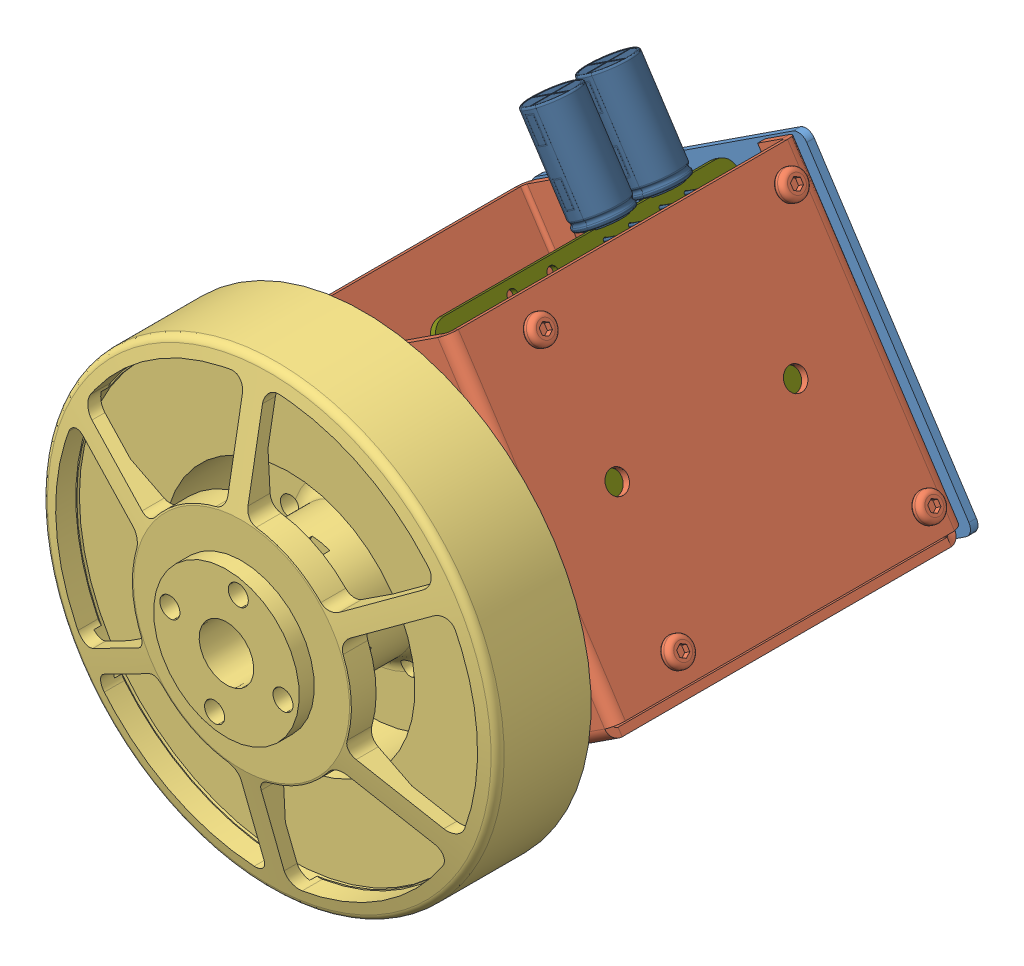
SolidWorks assembly 装配体1, configuration 默认. Lengths in mm.
Overall size (125.4 125.4 105.52).
333 component instances, 38 part files, 34 mates.
Components (placement in the parent):
- 后面板-1: 后面板 [默认] at (-110.0598 38.3936 -13.6207) x (-0.837169 -0.546944 0) z (0 0 -1) size (65 63 1.5)
- 电机架-钣金-1: 电机架-钣金 [默认] at (-110.4773 39.0327 57.0038) x (-0.837169 -0.546944 0) z (0.546944 -0.837169 0) size (65 70 63)
- bldc-motor-A12-1: bldc-motor-A12 [默认] at (-110.4773 39.0327 57.0038) x (-0.837169 -0.546944 0) z (-0.546944 0.837169 0) size (90.6 34.9 90.6)
- simple_bldc.step-1: simple_bldc.step [默认] at (-80.5102 22.4176 -12.7962) x (0 0 1) z (-0.837169 -0.546944 0) size (60.6 79.73 16.29)
  - JST_PH_B6B-PH-K_1x06_P2.00mm_Vertical.step-1: JST_PH_B6B-PH-K_1x06_P2.00mm_Vertical.step [默认] at (24 3 1.25) x (-1 0 0) z (0 0 1) size (13.9 4.55 9.4)
    - SOLID.step-1: SOLID.step [默认] at origin size (13.9 4.55 9.4)
  - SOT-363_SC-70-6.step-1: SOT-363_SC-70-6.step [默认] at (22.4536 8.4836 1.25) size (2 2 1.05)
    - SOLID-0.step-1: SOLID-0.step [默认] at origin size (2 2 1.05)
  - C_0402_1005Metric.step-1: C_0402_1005Metric.step [默认] at (10.668 38.1508 1.25) x (0 -1 0) z (0 0 1) size (1 0.5 0.5)
    - SOLID-1.step-1: SOLID-1.step [默认] at origin size (1 0.5 0.5)
  - PinHeader_1x06_P1.27mm_Vertical.step-1: PinHeader_1x06_P1.27mm_Vertical.step [默认] at (16.9418 25.5778 1.25) size (2.1 7.62 6.3)
    - SOLID-2.step-1: SOLID-2.step [默认] at origin size (2.1 7.62 6.3)
  - C_1206_3216Metric.step-1: C_1206_3216Metric.step [默认] at (7.75 37.6 1.25) size (3.2 1.6 1.6)
    - SOLID-3.step-1: SOLID-3.step [默认] at origin size (3.2 1.6 1.6)
  - LED_0603_1608Metric.step-1: LED_0603_1608Metric.step [默认] at (16.2574 49.0188 1.25) x (0 -1 0) z (0 0 1) size (1.6 0.8 1.1)
    - SOLID-4.step-1: SOLID-4.step [默认] at origin size (1.6 0.8 1.1)
  - SOIC-8_3.9x4.9mm_P1.27mm.step-1: SOIC-8_3.9x4.9mm_P1.27mm.step [默认] at (24.8434 32.3337 1.25) x (0 1 0) z (0 0 1) size (6 4.9 1.75)
    - SOLID-5.step-1: SOLID-5.step [默认] at origin size (6 4.9 1.75)
  - TO-252-5_TabPin3.step-1: TO-252-5_TabPin3.step [默认] at (11.55 45.55 1.25) x (0 1 0) z (0 0 1) size (9.9 6.5 2.32)
    - SOLID-6.step-1: SOLID-6.step [默认] at origin size (9.9 6.5 2.32)
  - R_0402_1005Metric.step-1: R_0402_1005Metric.step [默认] at (25.0698 27.559 1.25) x (0 1 0) z (0 0 1) size (1 0.5 0.35)
    - SOLID-7.step-1: SOLID-7.step [默认] at origin size (1 0.5 0.35)
  - R_0402_1005Metric.step-2: R_0402_1005Metric.step [默认] at (24.003 27.559 1.25) x (0 1 0) z (0 0 1) size (1 0.5 0.35)
    - SOLID-7.step-1: SOLID-7.step [默认] at origin size (1 0.5 0.35)
  - R_0402_1005Metric.step-3: R_0402_1005Metric.step [默认] at (16.2574 46.6188 1.25) x (0 -1 0) z (0 0 1) size (1 0.5 0.35)
    - SOLID-7.step-1: SOLID-7.step [默认] at origin size (1 0.5 0.35)
  - R_0402_1005Metric.step-4: R_0402_1005Metric.step [默认] at (21.3868 36.8046 1.25) size (1 0.5 0.35)
    - SOLID-7.step-1: SOLID-7.step [默认] at origin size (1 0.5 0.35)
  - R_0402_1005Metric.step-5: R_0402_1005Metric.step [默认] at (13.7 38.15 1.25) x (0 1 0) z (0 0 1) size (1 0.5 0.35)
    - SOLID-7.step-1: SOLID-7.step [默认] at origin size (1 0.5 0.35)
  - DFN-8-1EP_6x5mm_Pitch1.27mm.step-1: DFN-8-1EP_6x5mm_Pitch1.27mm.step [默认] at (18.0213 44.6278 -0.05) x (1 0 0) z (0 0 -1) size (6 4.9 1.1)
    - SOLID-8.step-1: SOLID-8.step [默认] at origin size (6 4.9 1.1)
  - PinHeader_1x03_P2.54mm_Vertical.step-1: PinHeader_1x03_P2.54mm_Vertical.step [默认] at (39.5 3 1.25) x (0 1 0) z (0 0 1) size (2.54 7.62 11.54)
    - SOLID-9.step-1: SOLID-9.step [默认] at origin size (2.54 7.62 11.54)
  - D_SOD-123.step-1: D_SOD-123.step [默认] at (20.9804 33.6677 1.25) x (0 -1 0) z (0 0 1) size (3.8 1.6 1.25)
    - SOLID-10.step-1: SOLID-10.step [默认] at origin size (3.8 1.6 1.25)
  - C_0603_1608Metric.step-1: C_0603_1608Metric.step [默认] at (24.003 36.7665 1.25) size (1.6 0.8 0.8)
    - SOLID-11.step-1: SOLID-11.step [默认] at origin size (1.6 0.8 0.8)
  - C_0402_1005Metric.step-2: C_0402_1005Metric.step [默认] at (21.5392 29.6672 1.25) x (0 -1 0) z (0 0 1) size (1 0.5 0.5)
    - SOLID-1.step-1: SOLID-1.step [默认] at origin size (1 0.5 0.5)
  - C_1206_3216Metric.step-2: C_1206_3216Metric.step [默认] at (3.1 37.6 1.25) x (-1 0 0) z (0 0 1) size (3.2 1.6 1.6)
    - SOLID-3.step-1: SOLID-3.step [默认] at origin size (3.2 1.6 1.6)
  - C_0603_1608Metric.step-2: C_0603_1608Metric.step [默认] at (33.3913 36.7634 1.25) size (1.6 0.8 0.8)
    - SOLID-11.step-1: SOLID-11.step [默认] at origin size (1.6 0.8 0.8)
  - C_0402_1005Metric.step-3: C_0402_1005Metric.step [默认] at (30.8413 29.5634 1.25) x (0 -1 0) z (0 0 1) size (1 0.5 0.5)
    - SOLID-1.step-1: SOLID-1.step [默认] at origin size (1 0.5 0.5)
  - R_0402_1005Metric.step-6: R_0402_1005Metric.step [默认] at (41.175 7.6905 1.25) x (-1 0 0) z (0 0 1) size (1 0.5 0.35)
    - SOLID-7.step-1: SOLID-7.step [默认] at origin size (1 0.5 0.35)
  - C_0603_1608Metric.step-3: C_0603_1608Metric.step [默认] at (15.0622 33.2068 1.25) x (-1 0 0) z (0 0 1) size (1.6 0.8 0.8)
    - SOLID-11.step-1: SOLID-11.step [默认] at origin size (1.6 0.8 0.8)
  - C_1206_3216Metric.step-3: C_1206_3216Metric.step [默认] at (1.95 32.15 1.25) x (0 1 0) z (0 0 1) size (3.2 1.6 1.6)
    - SOLID-3.step-1: SOLID-3.step [默认] at origin size (3.2 1.6 1.6)
  - C_1206_3216Metric.step-4: C_1206_3216Metric.step [默认] at (3.1 35.5 1.25) x (-1 0 0) z (0 0 1) size (3.2 1.6 1.6)
    - SOLID-3.step-1: SOLID-3.step [默认] at origin size (3.2 1.6 1.6)
  - C_0603_1608Metric.step-4: C_0603_1608Metric.step [默认] at (15.0622 31.7844 1.25) x (-1 0 0) z (0 0 1) size (1.6 0.8 0.8)
    - SOLID-11.step-1: SOLID-11.step [默认] at origin size (1.6 0.8 0.8)
  - DFN-8-1EP_6x5mm_Pitch1.27mm.step-2: DFN-8-1EP_6x5mm_Pitch1.27mm.step [默认] at (54.7116 46.99 1.25) x (0 1 0) z (0 0 1) size (6 4.9 1.1)
    - SOLID-8.step-1: SOLID-8.step [默认] at origin size (6 4.9 1.1)
  - DFN-8-1EP_6x5mm_Pitch1.27mm.step-3: DFN-8-1EP_6x5mm_Pitch1.27mm.step [默认] at (48.7172 46.99 1.25) x (0 -1 0) z (0 0 1) size (6 4.9 1.1)
    - SOLID-8.step-1: SOLID-8.step [默认] at origin size (6 4.9 1.1)
  - DFN-8-1EP_6x5mm_Pitch1.27mm.step-4: DFN-8-1EP_6x5mm_Pitch1.27mm.step [默认] at (41.0972 46.9392 1.25) x (0 1 0) z (0 0 1) size (6 4.9 1.1)
    - SOLID-8.step-1: SOLID-8.step [默认] at origin size (6 4.9 1.1)
  - DFN-8-1EP_6x5mm_Pitch1.27mm.step-5: DFN-8-1EP_6x5mm_Pitch1.27mm.step [默认] at (35.1028 46.9392 1.25) x (0 -1 0) z (0 0 1) size (6 4.9 1.1)
    - SOLID-8.step-1: SOLID-8.step [默认] at origin size (6 4.9 1.1)
  - DFN-8-1EP_6x5mm_Pitch1.27mm.step-6: DFN-8-1EP_6x5mm_Pitch1.27mm.step [默认] at (27.6352 46.9392 1.25) x (0 1 0) z (0 0 1) size (6 4.9 1.1)
    - SOLID-8.step-1: SOLID-8.step [默认] at origin size (6 4.9 1.1)
  - DFN-8-1EP_6x5mm_Pitch1.27mm.step-7: DFN-8-1EP_6x5mm_Pitch1.27mm.step [默认] at (21.6408 46.9392 1.25) x (0 -1 0) z (0 0 1) size (6 4.9 1.1)
    - SOLID-8.step-1: SOLID-8.step [默认] at origin size (6 4.9 1.1)
  - D_SMA.step-1: D_SMA.step [默认] at (15.3924 28.9904 1.25) size (5 2.7 2.22)
    - SOLID-12.step-1: SOLID-12.step [默认] at origin size (5 2.7 2.22)
  - JST_PH_B4B-PH-K_1x04_P2.00mm_Vertical.step-1: JST_PH_B4B-PH-K_1x04_P2.00mm_Vertical.step [默认] at (35 3 1.25) x (-1 0 0) z (0 0 1) size (9.9 4.55 9.4)
    - SOLID-13.step-1: SOLID-13.step [默认] at origin size (9.9 4.55 9.4)
  - SOT-23-6.step-1: SOT-23-6.step [默认] at (11.0744 16.6878 1.25) size (2.8 2.9 1.55)
    - SOLID-14.step-1: SOLID-14.step [默认] at origin size (2.8 2.9 1.55)
  - D_SOD-123.step-2: D_SOD-123.step [默认] at (6.55 10.55 1.25) size (3.8 1.6 1.25)
    - SOLID-10.step-1: SOLID-10.step [默认] at origin size (3.8 1.6 1.25)
  - PinSocket_1x02_P2.54mm_Vertical.step-1: PinSocket_1x02_P2.54mm_Vertical.step [默认] at (48.5 2.5 1.25) x (-1 0 0) z (0 0 1) size (2.54 5.08 10.1)
    - SOLID-15.step-1: SOLID-15.step [默认] at origin size (2.54 5.08 10.1)
  - R_0402_1005Metric.step-7: R_0402_1005Metric.step [默认] at (4.35 33.7 1.25) size (1 0.5 0.35)
    - SOLID-7.step-1: SOLID-7.step [默认] at origin size (1 0.5 0.35)
  - R_0402_1005Metric.step-8: R_0402_1005Metric.step [默认] at (20.5 11 1.25) size (1 0.5 0.35)
    - SOLID-7.step-1: SOLID-7.step [默认] at origin size (1 0.5 0.35)
  - SOIC-8_3.9x4.9mm_P1.27mm.step-2: SOIC-8_3.9x4.9mm_P1.27mm.step [默认] at (41.15 12.1279 1.25) x (0 -1 0) z (0 0 1) size (6 4.9 1.75)
    - SOLID-5.step-1: SOLID-5.step [默认] at origin size (6 4.9 1.75)
  - LQFP-64_10x10mm_P0.5mm.step-1: LQFP-64_10x10mm_P0.5mm.step [默认] at (28.698 16.1455 1.25) x (0 -1 0) z (0 0 1) size (12 12 1.5)
    - SOLID-16.step-1: SOLID-16.step [默认] at origin size (12 12 1.5)
  - SOT-23-6.step-2: SOT-23-6.step [默认] at (7.239 32.3432 1.25) x (-1 0 0) z (0 0 1) size (2.8 2.9 1.55)
    - SOLID-14.step-1: SOLID-14.step [默认] at origin size (2.8 2.9 1.55)
  - C_1206_3216Metric.step-5: C_1206_3216Metric.step [默认] at (37.8884 45.2528 -0.05) x (0 1 0) z (0 0 -1) size (3.2 1.6 1.6)
    - SOLID-3.step-1: SOLID-3.step [默认] at origin size (3.2 1.6 1.6)
  - C_1206_3216Metric.step-6: C_1206_3216Metric.step [默认] at (26.5939 45.2528 -0.05) x (0 1 0) z (0 0 -1) size (3.2 1.6 1.6)
    - SOLID-3.step-1: SOLID-3.step [默认] at origin size (3.2 1.6 1.6)
  - C_1206_3216Metric.step-7: C_1206_3216Metric.step [默认] at (51.0964 46.3704 -0.05) x (-1 0 0) z (0 0 -1) size (3.2 1.6 1.6)
    - SOLID-3.step-1: SOLID-3.step [默认] at origin size (3.2 1.6 1.6)
  - C_1206_3216Metric.step-8: C_1206_3216Metric.step [默认] at (30.9288 45.2528 -0.05) x (0 1 0) z (0 0 -1) size (3.2 1.6 1.6)
    - SOLID-3.step-1: SOLID-3.step [默认] at origin size (3.2 1.6 1.6)
  - C_1206_3216Metric.step-9: C_1206_3216Metric.step [默认] at (24.4264 45.2528 -0.05) x (0 1 0) z (0 0 -1) size (3.2 1.6 1.6)
    - SOLID-3.step-1: SOLID-3.step [默认] at origin size (3.2 1.6 1.6)
  - C_1206_3216Metric.step-10: C_1206_3216Metric.step [默认] at (51.0964 44.1352 -0.05) x (-1 0 0) z (0 0 -1) size (3.2 1.6 1.6)
    - SOLID-3.step-1: SOLID-3.step [默认] at origin size (3.2 1.6 1.6)
  - C_1206_3216Metric.step-11: C_1206_3216Metric.step [默认] at (42.2233 45.2528 -0.05) x (0 1 0) z (0 0 -1) size (3.2 1.6 1.6)
    - SOLID-3.step-1: SOLID-3.step [默认] at origin size (3.2 1.6 1.6)
  - C_1206_3216Metric.step-12: C_1206_3216Metric.step [默认] at (28.7613 45.2528 -0.05) x (0 1 0) z (0 0 -1) size (3.2 1.6 1.6)
    - SOLID-3.step-1: SOLID-3.step [默认] at origin size (3.2 1.6 1.6)
  - C_1206_3216Metric.step-13: C_1206_3216Metric.step [默认] at (40.0559 45.2528 -0.05) x (0 1 0) z (0 0 -1) size (3.2 1.6 1.6)
    - SOLID-3.step-1: SOLID-3.step [默认] at origin size (3.2 1.6 1.6)
  - C_1206_3216Metric.step-14: C_1206_3216Metric.step [默认] at (44.3908 45.2528 -0.05) x (0 1 0) z (0 0 -1) size (3.2 1.6 1.6)
    - SOLID-3.step-1: SOLID-3.step [默认] at origin size (3.2 1.6 1.6)
  - C_0402_1005Metric.step-4: C_0402_1005Metric.step [默认] at (25.4 24.3332 1.25) x (0 -1 0) z (0 0 1) size (1 0.5 0.5)
    - SOLID-1.step-1: SOLID-1.step [默认] at origin size (1 0.5 0.5)
  - C_1206_3216Metric.step-15: C_1206_3216Metric.step [默认] at (46.6852 41.0972 1.25) x (0 1 0) z (0 0 1) size (3.2 1.6 1.6)
    - SOLID-3.step-1: SOLID-3.step [默认] at origin size (3.2 1.6 1.6)
  - C_1206_3216Metric.step-16: C_1206_3216Metric.step [默认] at (33.2232 41.0464 1.25) x (0 1 0) z (0 0 1) size (3.2 1.6 1.6)
    - SOLID-3.step-1: SOLID-3.step [默认] at origin size (3.2 1.6 1.6)
  - C_1206_3216Metric.step-17: C_1206_3216Metric.step [默认] at (19.7104 41.0464 1.25) x (0 1 0) z (0 0 1) size (3.2 1.6 1.6)
    - SOLID-3.step-1: SOLID-3.step [默认] at origin size (3.2 1.6 1.6)
  - C_1206_3216Metric.step-18: C_1206_3216Metric.step [默认] at (49.008 41.12 1.25) x (0 1 0) z (0 0 1) size (3.2 1.6 1.6)
    - SOLID-3.step-1: SOLID-3.step [默认] at origin size (3.2 1.6 1.6)
  - C_1206_3216Metric.step-19: C_1206_3216Metric.step [默认] at (22.0076 41.0825 1.25) x (0 1 0) z (0 0 1) size (3.2 1.6 1.6)
    - SOLID-3.step-1: SOLID-3.step [默认] at origin size (3.2 1.6 1.6)
  - C_1206_3216Metric.step-20: C_1206_3216Metric.step [默认] at (35.4864 41.0708 1.25) x (0 1 0) z (0 0 1) size (3.2 1.6 1.6)
    - SOLID-3.step-1: SOLID-3.step [默认] at origin size (3.2 1.6 1.6)
  - R_0402_1005Metric.step-9: R_0402_1005Metric.step [默认] at (54.5846 36.7411 1.25) x (-1 0 0) z (0 0 1) size (1 0.5 0.35)
    - SOLID-7.step-1: SOLID-7.step [默认] at origin size (1 0.5 0.35)
  - R_0402_1005Metric.step-10: R_0402_1005Metric.step [默认] at (48.4378 36.7919 1.25) x (-1 0 0) z (0 0 1) size (1 0.5 0.35)
    - SOLID-7.step-1: SOLID-7.step [默认] at origin size (1 0.5 0.35)
  - R_0402_1005Metric.step-11: R_0402_1005Metric.step [默认] at (45.6184 36.7411 1.25) x (-1 0 0) z (0 0 1) size (1 0.5 0.35)
    - SOLID-7.step-1: SOLID-7.step [默认] at origin size (1 0.5 0.35)
  - R_0402_1005Metric.step-12: R_0402_1005Metric.step [默认] at (39.2684 36.7919 1.25) x (-1 0 0) z (0 0 1) size (1 0.5 0.35)
    - SOLID-7.step-1: SOLID-7.step [默认] at origin size (1 0.5 0.35)
  - R_0402_1005Metric.step-13: R_0402_1005Metric.step [默认] at (36.4871 36.7284 1.25) x (-1 0 0) z (0 0 1) size (1 0.5 0.35)
    - SOLID-7.step-1: SOLID-7.step [默认] at origin size (1 0.5 0.35)
  - R_0402_1005Metric.step-14: R_0402_1005Metric.step [默认] at (30.4165 36.8046 1.25) x (-1 0 0) z (0 0 1) size (1 0.5 0.35)
    - SOLID-7.step-1: SOLID-7.step [默认] at origin size (1 0.5 0.35)
  - SOIC-8_3.9x4.9mm_P1.27mm.step-3: SOIC-8_3.9x4.9mm_P1.27mm.step [默认] at (52.3494 32.3499 1.25) x (0 1 0) z (0 0 1) size (6 4.9 1.75)
    - SOLID-5.step-1: SOLID-5.step [默认] at origin size (6 4.9 1.75)
  - L_Bourns-SRN4018.step-1: L_Bourns-SRN4018.step [默认] at (11.4 32.8 1.25) size (4 4.09 1.8)
    - COMPOUND.step-1: COMPOUND.step [默认] at origin size (4 4.09 1.8)
  - D_SOD-123.step-3: D_SOD-123.step [默认] at (48.4886 33.6423 1.25) x (0 -1 0) z (0 0 1) size (3.8 1.6 1.25)
    - SOLID-10.step-1: SOLID-10.step [默认] at origin size (3.8 1.6 1.25)
  - D_SOD-123.step-4: D_SOD-123.step [默认] at (39.4208 33.6931 1.25) x (0 -1 0) z (0 0 1) size (3.8 1.6 1.25)
    - SOLID-10.step-1: SOLID-10.step [默认] at origin size (3.8 1.6 1.25)
  - D_SOD-123.step-5: D_SOD-123.step [默认] at (30.2641 33.7058 1.25) x (0 -1 0) z (0 0 1) size (3.8 1.6 1.25)
    - SOLID-10.step-1: SOLID-10.step [默认] at origin size (3.8 1.6 1.25)
  - SOIC-8_3.9x4.9mm_P1.27mm.step-4: SOIC-8_3.9x4.9mm_P1.27mm.step [默认] at (43.3324 32.3215 1.25) x (0 1 0) z (0 0 1) size (6 4.9 1.75)
    - SOLID-5.step-1: SOLID-5.step [默认] at origin size (6 4.9 1.75)
  - SOIC-8_3.9x4.9mm_P1.27mm.step-5: SOIC-8_3.9x4.9mm_P1.27mm.step [默认] at (34.1249 32.3342 1.25) x (0 1 0) z (0 0 1) size (6 4.9 1.75)
    - SOLID-5.step-1: SOLID-5.step [默认] at origin size (6 4.9 1.75)
  - SOIC-14_3.9x8.7mm_P1.27mm.step-1: SOIC-14_3.9x8.7mm_P1.27mm.step [默认] at (50.625 22.3111 1.25) x (-1 0 0) z (0 0 1) size (6 8.7 1.75)
    - SOLID-17.step-1: SOLID-17.step [默认] at origin size (6 8.7 1.75)
  - R_0402_1005Metric.step-15: R_0402_1005Metric.step [默认] at (27.2288 26.2382 1.25) x (0 -1 0) z (0 0 1) size (1 0.5 0.35)
    - SOLID-7.step-1: SOLID-7.step [默认] at origin size (1 0.5 0.35)
  - R_0402_1005Metric.step-16: R_0402_1005Metric.step [默认] at (46.863 29.6418 1.25) x (0 -1 0) z (0 0 1) size (1 0.5 0.35)
    - SOLID-7.step-1: SOLID-7.step [默认] at origin size (1 0.5 0.35)
  - R_0402_1005Metric.step-17: R_0402_1005Metric.step [默认] at (47.8028 29.6418 1.25) x (0 -1 0) z (0 0 1) size (1 0.5 0.35)
    - SOLID-7.step-1: SOLID-7.step [默认] at origin size (1 0.5 0.35)
  - R_0402_1005Metric.step-18: R_0402_1005Metric.step [默认] at (37.7063 29.6799 1.25) x (0 -1 0) z (0 0 1) size (1 0.5 0.35)
    - SOLID-7.step-1: SOLID-7.step [默认] at origin size (1 0.5 0.35)
  - R_0402_1005Metric.step-19: R_0402_1005Metric.step [默认] at (38.6588 29.6799 1.25) x (0 -1 0) z (0 0 1) size (1 0.5 0.35)
    - SOLID-7.step-1: SOLID-7.step [默认] at origin size (1 0.5 0.35)
  - R_0402_1005Metric.step-20: R_0402_1005Metric.step [默认] at (28.4734 29.5783 1.25) x (0 -1 0) z (0 0 1) size (1 0.5 0.35)
    - SOLID-7.step-1: SOLID-7.step [默认] at origin size (1 0.5 0.35)
  - R_0402_1005Metric.step-21: R_0402_1005Metric.step [默认] at (29.4513 29.591 1.25) x (0 -1 0) z (0 0 1) size (1 0.5 0.35)
    - SOLID-7.step-1: SOLID-7.step [默认] at origin size (1 0.5 0.35)
  - R_0402_1005Metric.step-22: R_0402_1005Metric.step [默认] at (45.5704 23.3271 1.25) x (-1 0 0) z (0 0 1) size (1 0.5 0.35)
    - SOLID-7.step-1: SOLID-7.step [默认] at origin size (1 0.5 0.35)
  - R_0402_1005Metric.step-23: R_0402_1005Metric.step [默认] at (45.5704 24.2415 1.25) x (-1 0 0) z (0 0 1) size (1 0.5 0.35)
    - SOLID-7.step-1: SOLID-7.step [默认] at origin size (1 0.5 0.35)
  - R_0402_1005Metric.step-24: R_0402_1005Metric.step [默认] at (55.6232 24.0665 1.25) size (1 0.5 0.35)
    - SOLID-7.step-1: SOLID-7.step [默认] at origin size (1 0.5 0.35)
  - R_0402_1005Metric.step-25: R_0402_1005Metric.step [默认] at (55.6232 24.9555 1.25) size (1 0.5 0.35)
    - SOLID-7.step-1: SOLID-7.step [默认] at origin size (1 0.5 0.35)
  - R_0402_1005Metric.step-26: R_0402_1005Metric.step [默认] at (36.8554 17.3736 1.25) x (-1 0 0) z (0 0 1) size (1 0.5 0.35)
    - SOLID-7.step-1: SOLID-7.step [默认] at origin size (1 0.5 0.35)
  - R_0402_1005Metric.step-27: R_0402_1005Metric.step [默认] at (45.5704 22.3619 1.25) x (-1 0 0) z (0 0 1) size (1 0.5 0.35)
    - SOLID-7.step-1: SOLID-7.step [默认] at origin size (1 0.5 0.35)
  - R_0402_1005Metric.step-28: R_0402_1005Metric.step [默认] at (45.5704 25.1559 1.25) x (-1 0 0) z (0 0 1) size (1 0.5 0.35)
    - SOLID-7.step-1: SOLID-7.step [默认] at origin size (1 0.5 0.35)
  - R_0402_1005Metric.step-29: R_0402_1005Metric.step [默认] at (55.626 23.1775 1.25) x (-1 0 0) z (0 0 1) size (1 0.5 0.35)
    - SOLID-7.step-1: SOLID-7.step [默认] at origin size (1 0.5 0.35)
  - R_0402_1005Metric.step-30: R_0402_1005Metric.step [默认] at (55.626 25.8699 1.25) x (-1 0 0) z (0 0 1) size (1 0.5 0.35)
    - SOLID-7.step-1: SOLID-7.step [默认] at origin size (1 0.5 0.35)
  - R_0402_1005Metric.step-31: R_0402_1005Metric.step [默认] at (45.5704 26.0731 1.25) size (1 0.5 0.35)
    - SOLID-7.step-1: SOLID-7.step [默认] at origin size (1 0.5 0.35)
  - R_0402_1005Metric.step-32: R_0402_1005Metric.step [默认] at (55.626 26.7589 1.25) x (-1 0 0) z (0 0 1) size (1 0.5 0.35)
    - SOLID-7.step-1: SOLID-7.step [默认] at origin size (1 0.5 0.35)
  - R_0402_1005Metric.step-33: R_0402_1005Metric.step [默认] at (55.626 20.4851 1.25) size (1 0.5 0.35)
    - SOLID-7.step-1: SOLID-7.step [默认] at origin size (1 0.5 0.35)
  - R_0402_1005Metric.step-34: R_0402_1005Metric.step [默认] at (55.6288 19.5933 1.25) size (1 0.5 0.35)
    - SOLID-7.step-1: SOLID-7.step [默认] at origin size (1 0.5 0.35)
  - R_0402_1005Metric.step-35: R_0402_1005Metric.step [默认] at (11.6 38.15 1.25) x (0 1 0) z (0 0 1) size (1 0.5 0.35)
    - SOLID-7.step-1: SOLID-7.step [默认] at origin size (1 0.5 0.35)
  - R_0402_1005Metric.step-36: R_0402_1005Metric.step [默认] at (4.3434 31.8606 1.25) x (-1 0 0) z (0 0 1) size (1 0.5 0.35)
    - SOLID-7.step-1: SOLID-7.step [默认] at origin size (1 0.5 0.35)
  - R_0402_1005Metric.step-37: R_0402_1005Metric.step [默认] at (55.626 21.3995 1.25) x (-1 0 0) z (0 0 1) size (1 0.5 0.35)
    - SOLID-7.step-1: SOLID-7.step [默认] at origin size (1 0.5 0.35)
  - R_0402_1005Metric.step-38: R_0402_1005Metric.step [默认] at (12.6 38.15 1.25) x (0 -1 0) z (0 0 1) size (1 0.5 0.35)
    - SOLID-7.step-1: SOLID-7.step [默认] at origin size (1 0.5 0.35)
  - R_0402_1005Metric.step-39: R_0402_1005Metric.step [默认] at (55.6288 18.7071 1.25) size (1 0.5 0.35)
    - SOLID-7.step-1: SOLID-7.step [默认] at origin size (1 0.5 0.35)
  - R_0402_1005Metric.step-40: R_0402_1005Metric.step [默认] at (4.3434 32.775 1.25) size (1 0.5 0.35)
    - SOLID-7.step-1: SOLID-7.step [默认] at origin size (1 0.5 0.35)
  - R_0402_1005Metric.step-41: R_0402_1005Metric.step [默认] at (55.6288 17.8181 1.25) x (-1 0 0) z (0 0 1) size (1 0.5 0.35)
    - SOLID-7.step-1: SOLID-7.step [默认] at origin size (1 0.5 0.35)
  - R_0402_1005Metric.step-42: R_0402_1005Metric.step [默认] at (45.5704 18.6817 1.25) x (-1 0 0) z (0 0 1) size (1 0.5 0.35)
    - SOLID-7.step-1: SOLID-7.step [默认] at origin size (1 0.5 0.35)
  - R_0402_1005Metric.step-43: R_0402_1005Metric.step [默认] at (45.5704 20.5613 1.25) size (1 0.5 0.35)
    - SOLID-7.step-1: SOLID-7.step [默认] at origin size (1 0.5 0.35)
  - R_0402_1005Metric.step-44: R_0402_1005Metric.step [默认] at (20.4724 20.7772 1.25) x (-1 0 0) z (0 0 1) size (1 0.5 0.35)
    - SOLID-7.step-1: SOLID-7.step [默认] at origin size (1 0.5 0.35)
  - R_0402_1005Metric.step-45: R_0402_1005Metric.step [默认] at (36.8554 16.4338 1.25) size (1 0.5 0.35)
    - SOLID-7.step-1: SOLID-7.step [默认] at origin size (1 0.5 0.35)
  - R_0402_1005Metric.step-46: R_0402_1005Metric.step [默认] at (14.6522 12.8757 1.25) x (0 1 0) z (0 0 1) size (1 0.5 0.35)
    - SOLID-7.step-1: SOLID-7.step [默认] at origin size (1 0.5 0.35)
  - R_0402_1005Metric.step-47: R_0402_1005Metric.step [默认] at (16.459 12.8757 1.25) x (0 1 0) z (0 0 1) size (1 0.5 0.35)
    - SOLID-7.step-1: SOLID-7.step [默认] at origin size (1 0.5 0.35)
  - R_0402_1005Metric.step-48: R_0402_1005Metric.step [默认] at (18.2556 12.8757 1.25) x (0 1 0) z (0 0 1) size (1 0.5 0.35)
    - SOLID-7.step-1: SOLID-7.step [默认] at origin size (1 0.5 0.35)
  - R_0402_1005Metric.step-49: R_0402_1005Metric.step [默认] at (14.18 16.2386 1.25) x (-1 0 0) z (0 0 1) size (1 0.5 0.35)
    - SOLID-7.step-1: SOLID-7.step [默认] at origin size (1 0.5 0.35)
  - R_0402_1005Metric.step-50: R_0402_1005Metric.step [默认] at (14.18 17.145 1.25) x (-1 0 0) z (0 0 1) size (1 0.5 0.35)
    - SOLID-7.step-1: SOLID-7.step [默认] at origin size (1 0.5 0.35)
  - R_0402_1005Metric.step-51: R_0402_1005Metric.step [默认] at (26.3144 24.3078 1.25) x (0 -1 0) z (0 0 1) size (1 0.5 0.35)
    - SOLID-7.step-1: SOLID-7.step [默认] at origin size (1 0.5 0.35)
  - R_0402_1005Metric.step-52: R_0402_1005Metric.step [默认] at (16.0528 38.1508 1.25) x (0 -1 0) z (0 0 1) size (1 0.5 0.35)
    - SOLID-7.step-1: SOLID-7.step [默认] at origin size (1 0.5 0.35)
  - HRO_TYPE-C-31-M-12.step-1: HRO_TYPE-C-31-M-12.step [默认] at (-0.6 22 1.25) x (0 -1 0) z (0 0 1) size (8.95 7.9 4.2)
    - SOLID-18.step-1: SOLID-18.step [默认] at origin size (6 4.32 0.61)
    - SOLID-19.step-1: SOLID-19.step [默认] at origin size (6.9 0.99 0.3)
    - SOLID-20.step-1: SOLID-20.step [默认] at origin size (8.95 6.5 3.7)
    - SOLID-21.step-1: SOLID-21.step [默认] at origin size (8.95 7.3 4.2)
  - C_0402_1005Metric.step-5: C_0402_1005Metric.step [默认] at (41.1904 16.4281 1.25) size (1 0.5 0.5)
    - SOLID-1.step-1: SOLID-1.step [默认] at origin size (1 0.5 0.5)
  - C_0402_1005Metric.step-6: C_0402_1005Metric.step [默认] at (34.036 22.2758 1.25) x (-1 0 0) z (0 0 1) size (1 0.5 0.5)
    - SOLID-1.step-1: SOLID-1.step [默认] at origin size (1 0.5 0.5)
  - C_0402_1005Metric.step-7: C_0402_1005Metric.step [默认] at (20.4724 18.8722 1.25) size (1 0.5 0.5)
    - SOLID-1.step-1: SOLID-1.step [默认] at origin size (1 0.5 0.5)
  - C_0402_1005Metric.step-8: C_0402_1005Metric.step [默认] at (20.4978 12.0142 1.25) size (1 0.5 0.5)
    - SOLID-1.step-1: SOLID-1.step [默认] at origin size (1 0.5 0.5)
  - C_0402_1005Metric.step-9: C_0402_1005Metric.step [默认] at (34.2392 9.8044 1.25) x (-1 0 0) z (0 0 1) size (1 0.5 0.5)
    - SOLID-1.step-1: SOLID-1.step [默认] at origin size (1 0.5 0.5)
  - C_0402_1005Metric.step-10: C_0402_1005Metric.step [默认] at (36.83 19.7866 1.25) x (-1 0 0) z (0 0 1) size (1 0.5 0.5)
    - SOLID-1.step-1: SOLID-1.step [默认] at origin size (1 0.5 0.5)
  - C_0402_1005Metric.step-11: C_0402_1005Metric.step [默认] at (28.448 26.2382 1.25) x (0 1 0) z (0 0 1) size (1 0.5 0.5)
    - SOLID-1.step-1: SOLID-1.step [默认] at origin size (1 0.5 0.5)
  - C_0402_1005Metric.step-12: C_0402_1005Metric.step [默认] at (24.4856 24.3332 1.25) x (0 -1 0) z (0 0 1) size (1 0.5 0.5)
    - SOLID-1.step-1: SOLID-1.step [默认] at origin size (1 0.5 0.5)
  - C_0402_1005Metric.step-13: C_0402_1005Metric.step [默认] at (28.448 24.3078 1.25) x (0 -1 0) z (0 0 1) size (1 0.5 0.5)
    - SOLID-1.step-1: SOLID-1.step [默认] at origin size (1 0.5 0.5)
  - C_0402_1005Metric.step-14: C_0402_1005Metric.step [默认] at (35.7632 26.2128 1.25) x (0 1 0) z (0 0 1) size (1 0.5 0.5)
    - SOLID-1.step-1: SOLID-1.step [默认] at origin size (1 0.5 0.5)
  - C_0402_1005Metric.step-15: C_0402_1005Metric.step [默认] at (34.2392 8.8646 1.25) size (1 0.5 0.5)
    - SOLID-1.step-1: SOLID-1.step [默认] at origin size (1 0.5 0.5)
  - C_0402_1005Metric.step-16: C_0402_1005Metric.step [默认] at (20.498 12.9455 1.25) x (-1 0 0) z (0 0 1) size (1 0.5 0.5)
    - SOLID-1.step-1: SOLID-1.step [默认] at origin size (1 0.5 0.5)
  - C_0603_1608Metric.step-5: C_0603_1608Metric.step [默认] at (51.689 36.7919 1.25) size (1.6 0.8 0.8)
    - SOLID-11.step-1: SOLID-11.step [默认] at origin size (1.6 0.8 0.8)
  - C_0402_1005Metric.step-17: C_0402_1005Metric.step [默认] at (49.1236 29.6164 1.25) x (0 -1 0) z (0 0 1) size (1 0.5 0.5)
    - SOLID-1.step-1: SOLID-1.step [默认] at origin size (1 0.5 0.5)
  - C_0603_1608Metric.step-6: C_0603_1608Metric.step [默认] at (42.672 36.7919 1.25) size (1.6 0.8 0.8)
    - SOLID-11.step-1: SOLID-11.step [默认] at origin size (1.6 0.8 0.8)
  - C_0402_1005Metric.step-18: C_0402_1005Metric.step [默认] at (44.148 23.7843 1.25) x (0 -1 0) z (0 0 1) size (1 0.5 0.5)
    - SOLID-1.step-1: SOLID-1.step [默认] at origin size (1 0.5 0.5)
  - C_0402_1005Metric.step-19: C_0402_1005Metric.step [默认] at (56.9976 24.4983 1.25) x (0 1 0) z (0 0 1) size (1 0.5 0.5)
    - SOLID-1.step-1: SOLID-1.step [默认] at origin size (1 0.5 0.5)
  - C_0402_1005Metric.step-20: C_0402_1005Metric.step [默认] at (40.0812 29.6799 1.25) x (0 -1 0) z (0 0 1) size (1 0.5 0.5)
    - SOLID-1.step-1: SOLID-1.step [默认] at origin size (1 0.5 0.5)
  - C_0402_1005Metric.step-21: C_0402_1005Metric.step [默认] at (44.1452 25.6159 1.25) x (0 1 0) z (0 0 1) size (1 0.5 0.5)
    - SOLID-1.step-1: SOLID-1.step [默认] at origin size (1 0.5 0.5)
  - C_0402_1005Metric.step-22: C_0402_1005Metric.step [默认] at (56.9976 26.3017 1.25) x (0 1 0) z (0 0 1) size (1 0.5 0.5)
    - SOLID-1.step-1: SOLID-1.step [默认] at origin size (1 0.5 0.5)
  - C_0402_1005Metric.step-23: C_0402_1005Metric.step [默认] at (55.626 22.2885 1.25) x (-1 0 0) z (0 0 1) size (1 0.5 0.5)
    - SOLID-1.step-1: SOLID-1.step [默认] at origin size (1 0.5 0.5)
  - C_0402_1005Metric.step-24: C_0402_1005Metric.step [默认] at (57.0004 20.0505 1.25) x (0 1 0) z (0 0 1) size (1 0.5 0.5)
    - SOLID-1.step-1: SOLID-1.step [默认] at origin size (1 0.5 0.5)
  - C_0402_1005Metric.step-25: C_0402_1005Metric.step [默认] at (4.3434 30.9462 1.25) x (-1 0 0) z (0 0 1) size (1 0.5 0.5)
    - SOLID-1.step-1: SOLID-1.step [默认] at origin size (1 0.5 0.5)
  - C_0402_1005Metric.step-26: C_0402_1005Metric.step [默认] at (56.9976 18.2499 1.25) x (0 -1 0) z (0 0 1) size (1 0.5 0.5)
    - SOLID-1.step-1: SOLID-1.step [默认] at origin size (1 0.5 0.5)
  - C_0603_1608Metric.step-7: C_0603_1608Metric.step [默认] at (7.6708 35.2388 1.25) size (1.6 0.8 0.8)
    - SOLID-11.step-1: SOLID-11.step [默认] at origin size (1.6 0.8 0.8)
  - C_0402_1005Metric.step-27: C_0402_1005Metric.step [默认] at (45.5504 19.5989 1.25) x (-1 0 0) z (0 0 1) size (1 0.5 0.5)
    - SOLID-1.step-1: SOLID-1.step [默认] at origin size (1 0.5 0.5)
  - C_0402_1005Metric.step-28: C_0402_1005Metric.step [默认] at (20.464 16.2206 1.25) size (1 0.5 0.5)
    - SOLID-1.step-1: SOLID-1.step [默认] at origin size (1 0.5 0.5)
  - C_0402_1005Metric.step-29: C_0402_1005Metric.step [默认] at (20.4724 19.8374 1.25) x (-1 0 0) z (0 0 1) size (1 0.5 0.5)
    - SOLID-1.step-1: SOLID-1.step [默认] at origin size (1 0.5 0.5)
  - C_0402_1005Metric.step-30: C_0402_1005Metric.step [默认] at (27.2542 24.3078 1.25) x (0 -1 0) z (0 0 1) size (1 0.5 0.5)
    - SOLID-1.step-1: SOLID-1.step [默认] at origin size (1 0.5 0.5)
  - D_SMA.step-2: D_SMA.step [默认] at (4.3 49.35 1.25) x (-1 0 0) z (0 0 1) size (5 2.7 2.22)
    - SOLID-12.step-1: SOLID-12.step [默认] at origin size (5 2.7 2.22)
  - cap_el_horizontal_d10_h20_pitch5_w0.6.step-1: cap_el_horizontal_d10_h20_pitch5_w0.6.step [默认] at (23.55 57.925 -3.5) x (0 -1 0) z (0 0 1) size (22.11 10.01 13.1)
    - SOLID-22.step-1: SOLID-22.step [默认] at origin size (22.11 10.01 13.1)
  - cap_el_horizontal_d10_h20_pitch5_w0.6.step-2: cap_el_horizontal_d10_h20_pitch5_w0.6.step [默认] at (12.4266 57.925 -3.5) x (0 -1 0) z (0 0 1) size (22.11 10.01 13.1)
    - SOLID-22.step-1: SOLID-22.step [默认] at origin size (22.11 10.01 13.1)
  - R_2512_6332Metric.step-1: R_2512_6332Metric.step [默认] at (40.8348 40.7918 1.25) size (6.3 3.2 0.6)
    - SOLID-23.step-1: SOLID-23.step [默认] at origin size (6.3 3.2 0.6)
  - R_2512_6332Metric.step-2: R_2512_6332Metric.step [默认] at (54.3476 40.8502 1.25) size (6.3 3.2 0.6)
    - SOLID-23.step-1: SOLID-23.step [默认] at origin size (6.3 3.2 0.6)
  - C_0603_1608Metric.step-8: C_0603_1608Metric.step [默认] at (11.176 25.663 1.25) x (0 -1 0) z (0 0 1) size (1.6 0.8 0.8)
    - SOLID-11.step-1: SOLID-11.step [默认] at origin size (1.6 0.8 0.8)
  - SOT-223.step-1: SOT-223.step [默认] at (5.9838 27.0848 1.25) x (-1 0 0) z (0 0 1) size (7 6.5 1.7)
    - SOLID-24.step-1: SOLID-24.step [默认] at origin size (7 6.5 1.7)
  - C_0603_1608Metric.step-9: C_0603_1608Metric.step [默认] at (11.176 28.6348 1.25) x (0 1 0) z (0 0 1) size (1.6 0.8 0.8)
    - SOLID-11.step-1: SOLID-11.step [默认] at origin size (1.6 0.8 0.8)
  - R_0603_1608Metric.step-1: R_0603_1608Metric.step [默认] at (17.5514 45.212 1.25) x (0 -1 0) z (0 0 1) size (1.6 0.8 0.45)
    - SOLID-25.step-1: SOLID-25.step [默认] at origin size (1.6 0.8 0.45)
  - LED_0603_1608Metric.step-2: LED_0603_1608Metric.step [默认] at (18.2556 9.8757 1.25) x (0 1 0) z (0 0 1) size (1.6 0.8 1.1)
    - SOLID-4.step-1: SOLID-4.step [默认] at origin size (1.6 0.8 1.1)
  - L_Bourns_SRN6045TA.step-1: L_Bourns_SRN6045TA.step [默认] at (4.1 43.3 1.25) x (0 -1 0) z (0 0 1) size (6 6 4.2)
    - SOLID-26.step-1: SOLID-26.step [默认] at origin size (6 6 4.2)
  - LED_0603_1608Metric.step-3: LED_0603_1608Metric.step [默认] at (14.6522 9.8757 1.25) x (0 1 0) z (0 0 1) size (1.6 0.8 1.1)
    - SOLID-4.step-1: SOLID-4.step [默认] at origin size (1.6 0.8 1.1)
  - Oscillator_SMD_EuroQuartz_XO53-4Pin_5.0x3.2mm.step-1: Oscillator_SMD_EuroQuartz_XO53-4Pin_5.0x3.2mm.step [默认] at (32.1232 25.2308 1.25) x (-1 0 0) z (0 0 1) size (5 3.2 1)
    - SOLID-27.step-1: SOLID-27.step [默认] at origin size (5 3.2 1)
  - LED_0603_1608Metric.step-4: LED_0603_1608Metric.step [默认] at (16.459 9.8757 1.25) x (0 1 0) z (0 0 1) size (1.6 0.8 1.1)
    - SOLID-4.step-1: SOLID-4.step [默认] at origin size (1.6 0.8 1.1)
  - R_2512_6332Metric.step-3: R_2512_6332Metric.step [默认] at (27.3204 40.7852 1.25) size (6.3 3.2 0.6)
    - SOLID-23.step-1: SOLID-23.step [默认] at origin size (6.3 3.2 0.6)
  - COMPOUND-28.step-1: COMPOUND-28.step [默认] at origin size (60 60 1.2)
- 传感器支架-1: 传感器支架 [默认] at (-110.4773 39.0327 55.5038) x (0.20522 0.978716 0) z (-0.978716 0.20522 0) size (50 4 50)
- M3铜柱-15mm-1: M3铜柱-15mm [默认] at (-98.0346 76.6661 -7.7962) x (0.383143 -0.58645 -0.713637) z (-0.390319 0.597434 -0.700516) size (5.37 21 4.74)
- M3铜柱-15mm-2: M3铜柱-15mm [默认] at (-70.6874 34.8076 42.2038) x (-0.131231 0.200866 -0.970789) z (-0.530967 0.812715 0.239934) size (5.37 21 4.74)
- M3铜柱-15mm-3: M3铜柱-15mm [默认] at (-98.0346 76.6661 42.2038) x (-0.131231 0.200866 -0.970789) z (-0.530967 0.812715 0.239934) size (5.37 21 4.74)
- M3铜柱-15mm-4: M3铜柱-15mm [默认] at (-70.6874 34.8076 -7.7962) x (0.131231 -0.200866 0.970789) z (0.530967 -0.812715 -0.239934) size (5.37 21 4.74)
- M3螺帽-1: M3螺帽 [默认] at (-113.6059 66.4929 -7.7962) x (0.525143 -0.8038 -0.279519) z (0.152881 -0.234005 0.96014) size (6.24 2.51 5.51)
- M3螺帽-2: M3螺帽 [默认] at (-86.2587 24.6345 42.2038) x (0.546944 -0.837169 0) z (0 0 1) size (6.24 2.51 5.51)
- M3螺帽-3: M3螺帽 [默认] at (-86.2587 24.6345 -7.7962) x (0.501591 -0.76775 -0.398705) z (0.218069 -0.333783 0.917079) size (6.24 2.51 5.51)
- M3螺帽-4: M3螺帽 [默认] at (-113.6059 66.4929 42.2038) x (0.53924 -0.825377 0.16725) z (-0.091476 0.140017 0.985915) size (6.24 2.51 5.51)
- M3螺丝-7.6mm-1: M3螺丝-7.6mm [默认] at (-74.1198 32.5652 42.2038) x (0.546944 -0.837169 0) z (0 0 1) size (5.3 7.6 5.3)
- M3螺丝-7.6mm-2: M3螺丝-7.6mm [默认] at (-101.467 74.4236 42.2038) x (0.546944 -0.837169 0) z (0 0 1) size (5.3 7.6 5.3)
- M3螺丝-7.6mm-3: M3螺丝-7.6mm [默认] at (-101.467 74.4236 -7.7962) x (0.546944 -0.837169 0) z (0 0 1) size (5.3 7.6 5.3)
- M3螺丝-7.6mm-4: M3螺丝-7.6mm [默认] at (-74.1198 32.5652 -7.7962) x (0.546944 -0.837169 0) z (0 0 1) size (5.3 7.6 5.3)
Mates (geometry in assembly coordinates):
- 同心1: concentric aligned: circle of 电机架-钣金-1; circle of bldc-motor-A12-1
- 同心3: concentric aligned: circle of 电机架-钣金-1; circle of bldc-motor-A12-1
- 重合1: coincident anti-aligned: plane of 电机架-钣金-1 through (-110.4773 39.0327 57.0038) normal (0 0 1); plane of bldc-motor-A12-1 through (-110.4773 39.0327 57.0038) normal (0 0 -1)
- 同心7: concentric aligned: circle of 后面板-1; circle of 电机架-钣金-1
- 同心8: concentric aligned: circle of 后面板-1; circle of 电机架-钣金-1
- 重合8: coincident aligned: circle of 电机架-钣金-1; circle of 传感器支架-1
- 重合9: coincident aligned: circle of 电机架-钣金-1; circle of 传感器支架-1
- 同心11: concentric anti-aligned: circle of 电机架-钣金-1; circle of M3铜柱-15mm-1
- 同心12: concentric aligned: circle of simple_bldc.step-1/COMPOUND-28.step-1; circle of M3铜柱-15mm-1
- 重合10: coincident anti-aligned: plane of simple_bldc.step-1/COMPOUND-28.step-1 through (-96.9185 47.5327 17.2038) normal (0.837169 0.546944 0); plane of M3铜柱-15mm-1 through (-110.5921 68.4619 -7.7962) normal (-0.837169 -0.546944 0)
- 同心13: concentric anti-aligned: circle of 电机架-钣金-1; circle of M3铜柱-15mm-2
- 同心14: concentric aligned: circle of simple_bldc.step-1/COMPOUND-28.step-1; circle of M3铜柱-15mm-2
- 重合11: coincident anti-aligned: plane of simple_bldc.step-1/COMPOUND-28.step-1 through (-96.9185 47.5327 17.2038) normal (0.837169 0.546944 0); plane of M3铜柱-15mm-2 through (-83.2449 26.6035 42.2038) normal (-0.837169 -0.546944 0)
- 同心15: concentric aligned: circle of simple_bldc.step-1/COMPOUND-28.step-1; circle of M3铜柱-15mm-3
- 重合12: coincident anti-aligned: plane of simple_bldc.step-1/COMPOUND-28.step-1 through (-96.9185 47.5327 17.2038) normal (0.837169 0.546944 0); plane of M3铜柱-15mm-3 through (-110.5921 68.4619 42.2038) normal (-0.837169 -0.546944 0)
- 同心16: concentric aligned: circle of simple_bldc.step-1/COMPOUND-28.step-1; circle of M3铜柱-15mm-4
- 重合13: coincident anti-aligned: plane of simple_bldc.step-1/COMPOUND-28.step-1 through (-96.9185 47.5327 17.2038) normal (0.837169 0.546944 0); plane of M3铜柱-15mm-4 through (-83.2449 26.6035 -7.7962) normal (-0.837169 -0.546944 0)
- 同心17: concentric anti-aligned: circle of M3铜柱-15mm-3; circle of M3螺帽-4
- 重合14: coincident anti-aligned: plane of simple_bldc.step-1/COMPOUND-28.step-1 through (-97.9231 46.8764 17.2038) normal (-0.837169 -0.546944 0); plane of M3螺帽-4 through (-111.5967 67.8056 42.2038) normal (0.837169 0.546944 0)
- 同心18: concentric anti-aligned: circle of M3铜柱-15mm-2; circle of M3螺帽-2
- 重合15: coincident anti-aligned: plane of simple_bldc.step-1/COMPOUND-28.step-1 through (-97.9231 46.8764 17.2038) normal (-0.837169 -0.546944 0); plane of M3螺帽-2 through (-84.2495 25.9471 42.2038) normal (0.837169 0.546944 0)
- 同心19: concentric anti-aligned: circle of M3铜柱-15mm-1; circle of M3螺帽-1
- 重合16: coincident anti-aligned: plane of simple_bldc.step-1/COMPOUND-28.step-1 through (-97.9231 46.8764 17.2038) normal (-0.837169 -0.546944 0); plane of M3螺帽-1 through (-111.5967 67.8056 -7.7962) normal (0.837169 0.546944 0)
- 同心20: concentric anti-aligned: circle of M3铜柱-15mm-4; circle of M3螺帽-3
- 重合17: coincident anti-aligned: plane of simple_bldc.step-1/COMPOUND-28.step-1 through (-97.9231 46.8764 17.2038) normal (-0.837169 -0.546944 0); plane of M3螺帽-3 through (-84.2495 25.9471 -7.7962) normal (0.837169 0.546944 0)
- 重合19: coincident anti-aligned: plane of 电机架-钣金-1 through (-84.5251 55.988 57.0038) normal (-0.837169 -0.546944 0); plane of M3铜柱-15mm-3 through (-98.0346 76.6661 42.2038) normal (0.837169 0.546944 0)
- 同心21: concentric aligned: circle of 电机架-钣金-1; circle of M3螺丝-7.6mm-4
- 重合20: coincident anti-aligned: plane of 电机架-钣金-1 through (-83.2693 56.8084 57.0038) normal (0.837169 0.546944 0); plane of M3螺丝-7.6mm-4 through (-70.252 36.8838 -7.7962) normal (-0.837169 -0.546944 0)
- 同心22: concentric anti-aligned: circle of 电机架-钣金-1; circle of M3螺丝-7.6mm-1
- 重合21: coincident anti-aligned: plane of 电机架-钣金-1 through (-83.2693 56.8084 57.0038) normal (0.837169 0.546944 0); plane of M3螺丝-7.6mm-1 through (-70.252 36.8838 42.2038) normal (-0.837169 -0.546944 0)
- 同心23: concentric anti-aligned: circle of 电机架-钣金-1; circle of M3螺丝-7.6mm-2
- 重合22: coincident anti-aligned: plane of 电机架-钣金-1 through (-83.2693 56.8084 57.0038) normal (0.837169 0.546944 0); plane of M3螺丝-7.6mm-2 through (-97.5992 78.7423 42.2038) normal (-0.837169 -0.546944 0)
- 同心24: concentric anti-aligned: circle of 电机架-钣金-1; circle of M3螺丝-7.6mm-3
- 重合23: coincident anti-aligned: plane of 电机架-钣金-1 through (-83.2693 56.8084 57.0038) normal (0.837169 0.546944 0); plane of M3螺丝-7.6mm-3 through (-97.5992 78.7423 -7.7962) normal (-0.837169 -0.546944 0)
